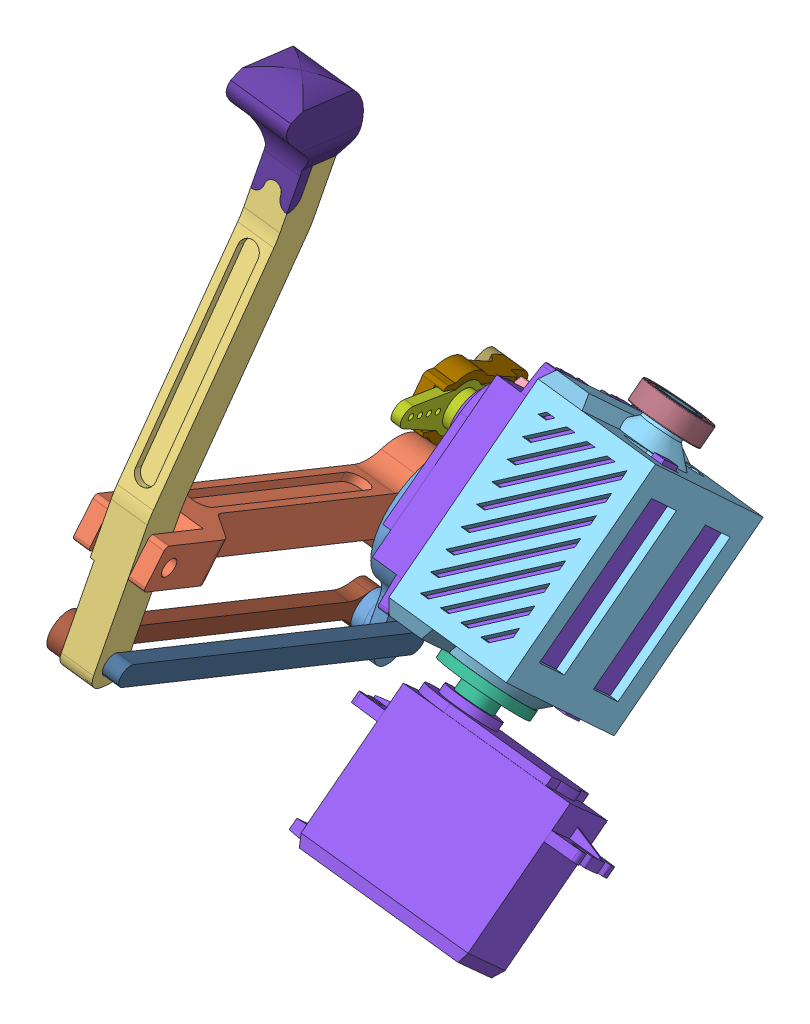
SolidWorks assembly Leg 1, configuration Default. Lengths in mm.
Overall size (88.68 208.64 144.57).
30 component instances, 17 part files, 41 mates.
Components (placement in the parent):
- RearRotatingPiece-1: RearRotatingPiece [Default] at (-127.382 103.5441 89.0438) x (0.203985 0.956422 0.20892) z (-0.017219 0.216879 -0.976047) size (44.28 13.7 43.21)
- RearUpperLeg-1: RearUpperLeg [Default] at (-114.3555 145.7963 184.4224) x (-0.14634 -0.875618 0.460302) z (0.978823 -0.195502 -0.060709) size (22 116.4 18)
- RearLowerLeg-1: RearLowerLeg [Default] at (-93.707 239.8256 140.4142) x (-0.102671 -0.212274 -0.971802) z (-0.978823 0.195502 0.060709) size (20.21 126 9.59)
- RearShortConnectingRod-1: RearShortConnectingRod [Default] at (-185.9448 141.3093 79.0671) x (-0.202239 -0.969447 -0.13882) z (-0.978823 0.195502 0.060709) size (37.08 6.33 13)
- RearServoHousing-2: RearServoHousing [Default] at (-144.3175 82.1208 49.6998) x (0.098774 0.710794 -0.696431) z (-0.978823 0.195502 0.060709) size (61.5 52 29.25)
- Circle Rudder-1: Circle Rudder [默认] at (-120.1327 99.362 109.8548) x (-0.707237 0.542477 0.453358) z (0.700042 0.447762 0.556282) size (20.8 5.5 20.8)
- Double_Blade_Rudder-1: Double_Blade_Rudder [默认] at (-145.4785 141.5037 95.0658) x (0.153804 0.898037 -0.412157) z (-0.135096 -0.394091 -0.909088) size (12.2 5.5 38)
- Circle Rudder-2: Circle Rudder [默认] at (-152.1463 108.4903 90.5797) x (-0.142725 -0.864334 0.482241) z (0.146752 0.463364 0.873933) size (20.8 5.5 20.8)
- MG996R-4: MG996R [Default] at (-102.2058 125.2624 99.7037) x (-0.098774 -0.710794 0.696431) z (-0.179305 -0.675686 -0.715051) size (54.5 42.75 20)
- MG996R-5: MG996R [Default] at (-107.0313 107.0778 80.4598) x (0.098774 0.710794 -0.696431) z (0.179305 0.675686 0.715051) size (54.5 42.75 20)
- Servo Arm Mount-1: Servo Arm Mount [Default] at (-145.5764 141.5232 95.0719) x (0.153804 0.898037 -0.412157) z (-0.978823 0.195502 0.060709) size (16.2 34.39 10.1)
- MG996R-6: MG996R [Default] at (-114.4434 64.8451 140.1199) x (0.967861 -0.231274 -0.098774) z (0.231274 0.664293 0.710794) size (54.5 42.75 20)
- Long Connecting Rod-1: Long Connecting Rod [Default] at (-141.9668 132.2907 186.2965) x (0.143149 0.44168 0.885679) z (0.978823 -0.195502 -0.060709) size (105.4 5 16.7)
- Long Connecting Rod Alt-1: Long Connecting Rod Alt [Default] at (-150.5211 130.5615 185.7188) x (0.143149 0.44168 0.885679) z (-0.146338 -0.875613 0.460313) size (109.5 4 9.1)
- Short Connecting Rod Alt-1: Short Connecting Rod Alt [Default] at (-160.8016 101.1459 70.217) x (-0.202239 -0.969447 -0.13882) z (-0.031714 0.148158 -0.988455) size (41.18 3 8.1)
- 688ZZ Bearing Assembly-2: 688ZZ Bearing Assembly [Default] at (-114.3051 141.2989 68.7654) x (0.967861 -0.231274 -0.098774) z (0.098774 0.710794 -0.696431) size (17.99 17.98 5)
  - Outer Ring-1: Outer Ring [Default] at origin size (16 16 5)
  - Inner Ring-1: Inner Ring [Default] x (-0.241565 -0.970385 0) z (0 0 1) size (10.6 10.6 5)
  - Cage-1: Cage [Default] x (0.535517 0.844524 0) z (0 0 1) size (13.01 13.06 2.21)
  - 2mm Ball Bearing-1: 2mm Ball Bearing [Default] at (-5.0671 3.2131 0) x (0.050652 0.835774 0.546732) z (0.977207 -0.154478 0.145614) size (2 2 2)
  - 2mm Ball Bearing-2: 2mm Ball Bearing [Default] at (-5.988 -0.3789 0) x (-0.450278 0.705928 0.546732) z (0.881377 0.449412 0.145614) size (2 2 2)
  - 2mm Ball Bearing-3: 2mm Ball Bearing [Default] at (-4.6217 -3.8262 0) x (-0.779216 0.306441 0.546732) z (0.448891 0.881642 0.145614) size (2 2 2)
  - 2mm Ball Bearing-4: 2mm Ball Bearing [Default] at (-1.49 -5.812 0) x (-0.810521 -0.210096 0.546732) z (-0.155056 0.977115 0.145614) size (2 2 2)
  - 2mm Ball Bearing-5: 2mm Ball Bearing [Default] at (2.2108 -5.5778 0) x (-0.532234 -0.646383 0.546732) z (-0.699777 0.699363 0.145614) size (2 2 2)
  - 2mm Ball Bearing-6: 2mm Ball Bearing [Default] at (5.0671 -3.2131 0) x (-0.050652 -0.835774 0.546732) z (-0.977207 0.154478 0.145614) size (2 2 2)
  - 2mm Ball Bearing-7: 2mm Ball Bearing [Default] at (5.988 0.3789 0) x (0.450278 -0.705928 0.546732) z (-0.881377 -0.449412 0.145614) size (2 2 2)
  - 2mm Ball Bearing-8: 2mm Ball Bearing [Default] at (4.6217 3.8262 0) x (0.779216 -0.306441 0.546732) z (-0.448891 -0.881642 0.145614) size (2 2 2)
  - 2mm Ball Bearing-9: 2mm Ball Bearing [Default] at (1.49 5.812 0) x (0.810521 0.210096 0.546732) z (0.155056 -0.977115 0.145614) size (2 2 2)
  - 2mm Ball Bearing-10: 2mm Ball Bearing [Default] at (-2.2108 5.5778 0) x (0.532234 0.646383 0.546732) z (0.699777 -0.699363 0.145614) size (2 2 2)
- Foot Cap R2-1: Foot Cap R2 [Default] at (-122.0928 245.4951 142.1747) x (-0.102671 -0.212274 -0.971802) z (-0.978823 0.195502 0.060709) size (26.22 31.5 15)
Mates (geometry in assembly coordinates):
- Concentric7: concentric anti-aligned: circle of Circle Rudder-1; circle of RearServoHousing-2
- Coincident15: coincident anti-aligned: plane of RearServoHousing-2 through (-35.9087 73.2904 95.1908) normal (-0.098774 -0.710794 0.696431); plane of Circle Rudder-1 through (-120.1327 99.362 109.8548) normal (0.098774 0.710794 -0.696431)
- Concentric8: concentric aligned: cylinder of MG996R-5 through (-137.0292 91.4112 96.1128) axis (-0.978823 0.195502 0.060709) radius 1.7678; cylinder of RearServoHousing-2 through (-129.1986 89.8472 95.6271) axis (-0.978823 0.195502 0.060709) radius 0.7
- Coincident16: coincident anti-aligned: plane of RearServoHousing-2 through (-106.9495 107.3862 80.7861) normal (-0.978823 0.195502 0.060709); plane of MG996R-5 through (-107.0313 107.0778 80.4598) normal (0.978823 -0.195502 -0.060709)
- Concentric9: concentric anti-aligned: cylinder of MG996R-5 through (-130.2975 133.7077 68.4418) axis (-0.978823 0.195502 0.060709) radius 1.7678; circle of RearServoHousing-2
- Concentric10: concentric anti-aligned: cylinder of MG996R-4 through (-127.3468 144.827 80.2089) axis (-0.978823 0.195502 0.060709) radius 1.7678; circle of RearServoHousing-2
- Coincident17: coincident anti-aligned: plane of RearServoHousing-2 through (-106.9495 107.3862 80.7861) normal (-0.978823 0.195502 0.060709); plane of MG996R-4 through (-102.2058 125.2624 99.7037) normal (0.978823 -0.195502 -0.060709)
- Parallel2: parallel anti-aligned: plane of MG996R-4 through (-133.4055 153.402 94.9219) normal (0.179305 0.675686 0.715051); plane of RearServoHousing-2 through (-26.7622 116.9842 101.9549) normal (-0.179305 -0.675686 -0.715051)
- Concentric12: concentric aligned: cylinder of Circle Rudder-2 through (-149.895 108.0407 90.4401) axis (-0.978823 0.195502 0.060709) radius 1.5; cylinder of MG996R-5 through (-146.9585 107.4542 90.258) axis (-0.978823 0.195502 0.060709) radius 1.5
- Coincident20: coincident anti-aligned: plane of Circle Rudder-2 through (-149.895 108.0407 90.4401) normal (0.978823 -0.195502 -0.060709); plane of MG996R-5 through (-149.895 108.0407 90.4401) normal (-0.978823 0.195502 0.060709)
- Coincident21: coincident anti-aligned: plane of RearUpperLeg-1 through (-152.1463 108.4903 90.5797) normal (0.978823 -0.195502 -0.060709); plane of Circle Rudder-2 through (-152.1463 108.4903 90.5797) normal (-0.978823 0.195502 0.060709)
- Concentric13: concentric anti-aligned: cylinder of RearUpperLeg-1 through (-160.9557 110.2499 91.1261) axis (0.978823 -0.195502 -0.060709) radius 1.7; cylinder of Circle Rudder-2 through (-149.895 108.0407 90.4401) axis (-0.978823 0.195502 0.060709) radius 1.5
- Concentric14: concentric anti-aligned: cylinder of RearRotatingPiece-1 through (-148.9161 107.8452 90.3794) axis (0.978823 -0.195502 -0.060709) radius 4.35; cylinder of Circle Rudder-2 through (-146.7627 107.4151 90.2458) axis (-0.978823 0.195502 0.060709) radius 4.4
- Coincident22: coincident anti-aligned: plane of RearRotatingPiece-1 through (-146.9585 107.4542 90.258) normal (0.978823 -0.195502 -0.060709); plane of MG996R-5 through (-146.9585 107.4542 90.258) normal (-0.978823 0.195502 0.060709)
- Concentric16: concentric aligned: cylinder of Double_Blade_Rudder-1 through (-143.2272 141.054 94.9262) axis (-0.978823 0.195502 0.060709) radius 1.5; cylinder of MG996R-4 through (-140.095 140.4284 94.7319) axis (-0.978823 0.195502 0.060709) radius 1.5
- Coincident24: coincident anti-aligned: plane of Double_Blade_Rudder-1 through (-140.095 140.4284 94.7319) normal (0.978823 -0.195502 -0.060709); plane of MG996R-4 through (-140.095 140.4284 94.7319) normal (-0.978823 0.195502 0.060709)
- Concentric18: concentric aligned: cylinder of RearRotatingPiece-1 through (-158.7461 100.7353 70.0895) axis (0.978823 -0.195502 -0.060709) radius 2.2; cylinder of RearShortConnectingRod-1 through (-164.7169 101.9279 70.4599) axis (0.978823 -0.195502 -0.060709) radius 2
- Concentric19: concentric anti-aligned: cylinder of RearShortConnectingRod-1 through (-157.9257 134.4819 75.1214) axis (0.978823 -0.195502 -0.060709) radius 1.5; cylinder of Servo Arm Mount-1 through (-144.418 131.784 74.2836) axis (-0.978823 0.195502 0.060709) radius 1.7
- Concentric20: concentric anti-aligned: cylinder of Double_Blade_Rudder-1 through (-143.2272 141.054 94.9262) axis (-0.978823 0.195502 0.060709) radius 1.5; cylinder of Servo Arm Mount-1 through (-148.5129 142.1097 95.254) axis (0.978823 -0.195502 -0.060709) radius 1.7
- Concentric21: concentric aligned: cylinder of RearUpperLeg-1 through (-133.8583 152.0541 179.2637) axis (-0.978823 0.195502 0.060709) radius 2.1; cylinder of RearLowerLeg-1 through (-138.263 152.9338 179.5369) axis (-0.978823 0.195502 0.060709) radius 2
- Concentric22: concentric aligned: cylinder of Circle Rudder-1 through (-120.676 95.4527 113.6852) axis (0.098774 0.710794 -0.696431) radius 3; cylinder of MG996R-6 through (-120.6562 95.5948 113.5459) axis (0.098774 0.710794 -0.696431) radius 1.5
- Coincident39: coincident anti-aligned: plane of Circle Rudder-1 through (-120.3599 97.7272 111.4566) normal (-0.098774 -0.710794 0.696431); plane of MG996R-6 through (-120.3599 97.7272 111.4566) normal (0.098774 0.710794 -0.696431)
- Concentric23: concentric anti-aligned: cylinder of RearRotatingPiece-1 through (-160.195 85.2783 96.5053) axis (0.978823 -0.195502 -0.060709) radius 2.7; cylinder of Long Connecting Rod-1 through (-153.1474 83.8707 96.0682) axis (-0.978823 0.195502 0.060709) radius 2.5
- Concentric24: concentric aligned: cylinder of RearLowerLeg-1 through (-142.6905 128.9975 185.2331) axis (-0.978823 0.195502 0.060709) radius 2.6; cylinder of Long Connecting Rod-1 through (-138.7752 128.2154 184.9903) axis (-0.978823 0.195502 0.060709) radius 2.5
- Coincident40: coincident anti-aligned: plane of RearRotatingPiece-1 through (-155.7191 100.2702 67.6806) normal (0.978823 -0.195502 -0.060709); plane of Long Connecting Rod-1 through (-141.9668 132.2907 186.2965) normal (-0.978823 0.195502 0.060709)
- Concentric25: concentric anti-aligned: cylinder of Long Connecting Rod-1 through (-153.1474 83.8707 96.0682) axis (-0.978823 0.195502 0.060709) radius 2.5; cylinder of Long Connecting Rod Alt-1 through (-168.8086 86.9988 97.0395) axis (0.978823 -0.195502 -0.060709) radius 2.55
- Concentric26: concentric anti-aligned: cylinder of Long Connecting Rod-1 through (-138.7752 128.2154 184.9903) axis (-0.978823 0.195502 0.060709) radius 2.5; cylinder of Long Connecting Rod Alt-1 through (-154.4364 131.3435 185.9616) axis (0.978823 -0.195502 -0.060709) radius 2.55
- Coincident42: coincident anti-aligned: plane of RearLowerLeg-1 through (-150.8933 126.8356 191.7171) normal (-0.978823 0.195502 0.060709); plane of Long Connecting Rod Alt-1 through (-150.5211 130.5615 185.7188) normal (0.978823 -0.195502 -0.060709)
- Distance2: distance = 0.5 mm anti-aligned: plane of RearLowerLeg-1 through (-122.0928 245.4951 142.1747) normal (0.978823 -0.195502 -0.060709); plane of RearUpperLeg-1 through (-131.9815 185.5859 167.429) normal (-0.978823 0.195502 0.060709)
- Concentric27: concentric anti-aligned: cylinder of Double_Blade_Rudder-1 through (-143.2272 141.054 94.9262) axis (-0.978823 0.195502 0.060709) radius 1.5; cylinder of Servo Arm Mount-1 through (-148.5129 142.1097 95.254) axis (0.978823 -0.195502 -0.060709) radius 1.7
- Coincident44: coincident anti-aligned: plane of Double_Blade_Rudder-1 through (-145.4785 141.5037 95.0658) normal (-0.978823 0.195502 0.060709); plane of Servo Arm Mount-1 through (-145.4785 141.5037 95.0658) normal (0.978823 -0.195502 -0.060709)
- Concentric28: concentric aligned: cylinder of Double_Blade_Rudder-1 through (-144.1729 138.2954 88.5626) axis (-0.978823 0.195502 0.060709) radius 0.75; cylinder of Servo Arm Mount-1 through (-146.4242 138.745 88.7022) axis (-0.978823 0.195502 0.060709) radius 0.75
- Concentric29: concentric anti-aligned: cylinder of RearShortConnectingRod-1 through (-157.9257 134.4819 75.1214) axis (0.978823 -0.195502 -0.060709) radius 1.5; cylinder of Servo Arm Mount-1 through (-144.418 131.784 74.2836) axis (-0.978823 0.195502 0.060709) radius 1.7
- Coincident45: coincident anti-aligned: plane of RearShortConnectingRod-1 through (-154.8038 126.6737 2.3531) normal (-0.978823 0.195502 0.060709); plane of Servo Arm Mount-1 through (-149.1163 132.7224 74.575) normal (0.978823 -0.195502 -0.060709)
- Concentric30: concentric aligned: cylinder of RearShortConnectingRod-1 through (-157.9257 134.4819 75.1214) axis (0.978823 -0.195502 -0.060709) radius 1.5; cylinder of Short Connecting Rod Alt-1 through (-156.9469 134.2864 75.0607) axis (0.978823 -0.195502 -0.060709) radius 1.55
- Concentric31: concentric aligned: cylinder of RearShortConnectingRod-1 through (-164.7169 101.9279 70.4599) axis (0.978823 -0.195502 -0.060709) radius 2; cylinder of Short Connecting Rod Alt-1 through (-163.7381 101.7324 70.3991) axis (0.978823 -0.195502 -0.060709) radius 2.05
- Concentric33: concentric anti-aligned: cylinder of RearServoHousing-2 through (-114.0581 143.0759 67.0243) axis (-0.098774 -0.710794 0.696431) radius 4; cylinder of 688ZZ Bearing Assembly-2/Inner Ring-1 through (-113.6378 146.1006 64.0607) axis (0.098774 0.710794 -0.696431) radius 4
- Coincident47: coincident anti-aligned: plane of RearServoHousing-2 through (-114.552 139.5219 70.5065) normal (0.098774 0.710794 -0.696431); plane of 688ZZ Bearing Assembly-2/Inner Ring-1 through (-109.4274 139.1925 70.8971) normal (-0.098774 -0.710794 0.696431)
- Coincident48: coincident anti-aligned: plane of RearRotatingPiece-1 through (-157.8234 109.6242 90.9318) normal (-0.978823 0.195502 0.060709); plane of Short Connecting Rod Alt-1 through (-160.8016 101.1459 70.217) normal (0.978823 -0.195502 -0.060709)
- Concentric34: concentric aligned: cylinder of RearLowerLeg-1 through (-129.7919 226.851 152.2057) axis (0.102671 0.212274 0.971802) radius 2; cylinder of Foot Cap R2-1 through (-129.7919 226.851 152.2057) axis (0.102671 0.212274 0.971802) radius 2
- Concentric35: concentric anti-aligned: cylinder of RearLowerLeg-1 through (-131.4515 242.5713 148.9472) axis (0.978823 -0.195502 -0.060709) radius 2; cylinder of Foot Cap R2-1 through (-122.6421 240.8118 148.4008) axis (-0.978823 0.195502 0.060709) radius 2
